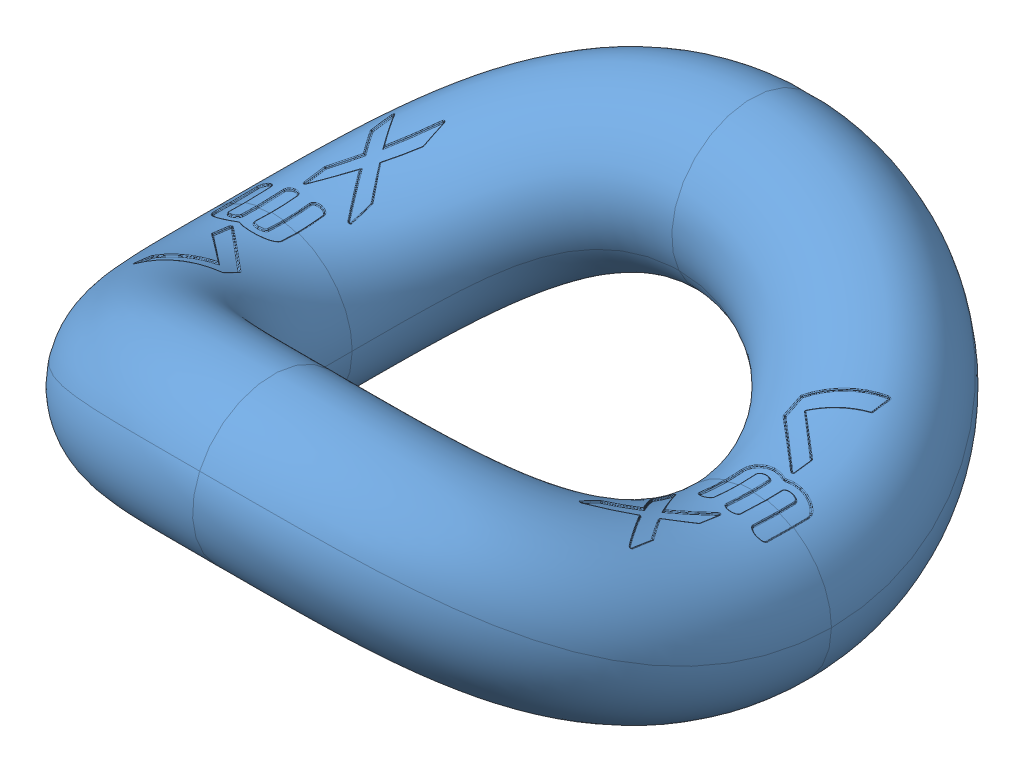
SolidWorks assembly Ring, configuration Default. Lengths in mm.
Overall size (101.61 43.55 104.58).
4 component instances, 1 part files, 0 mates.
Components (placement in the parent):
- Ring.step-1: Ring.step [Default] at origin size (101.61 43.55 104.58)
  - 276-7048-350 Rev2.step-1: 276-7048-350 Rev2.step [Default] at (-27.7593 -20.073 1639.1281) size (101.61 43.55 104.58)
    - 276-7048-301 Rev2 (1).step-1: 276-7048-301 Rev2 (1).step [Default] at (0 0 -1197.0106) x (0 0 -1) z (1 0 0) size (104.58 43.55 101.61)
      - 276-7048-001 Rev2.step-1: 276-7048-001 Rev2.step [Default] at (442.1175 9.4315 0) size (104.58 43.55 101.61)
